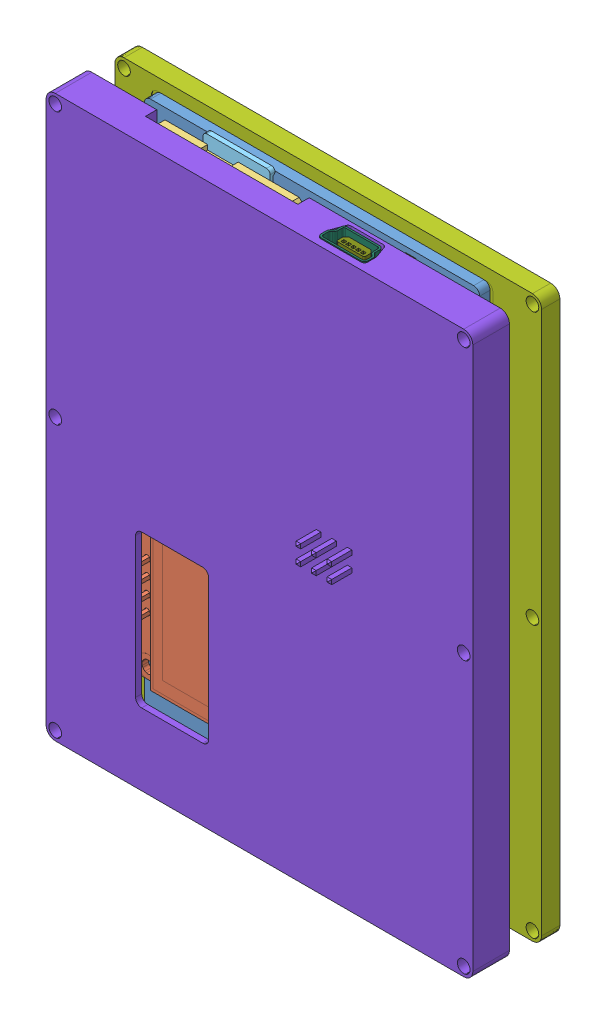
SolidWorks assembly Temperature & Humidity Meter, configuration Default. Lengths in mm.
Overall size (70.59 92.15 18.6).
51 component instances, 27 part files, 4 mates.
Components (placement in the parent):
- PCB.step-1: PCB.step [Default] at (27.42 35.7592 77.8723) size (55 92.15 18.6)
  - Board.step-1: Board.step [Default] at origin size (55 90 1.69)
    - Open CASCADE STEP translator 6.8 1.1.1.step-1: Open CASCADE STEP translator 6.8 1.1.1.step [Default] at (0 0 -1.6914) size (55 90 1.69)
  - O1.step-1: O1.step [Default] at origin size (27.98 26.7 10.85)
    - OLED_Display.step-1: OLED_Display.step [Default] at (-17.7739 15.5603 3.5437) x (0 1 0) z (0 0 1) size (26.7 27.98 10.85)
  - M1.step-1: M1.step [Default] at origin size (24 46.9 6.7)
    - MicroSD_Card.step-1: MicroSD_Card.step [Default] at (-7.7199 19.6 1.2127) x (0 -1 0) z (0 0 -1) size (46.9 24 6.7)
      - sdreader.step-1: sdreader.step [Default] at (-11.2744 2.632 -3.2) size (46.9 24 6.7)
        - Open CASCADE STEP translator 6.8 1.3.1.1.1.step-1: Open CASCADE STEP translator 6.8 1.3.1.1.1.step [Default] at origin size (46.9 24 6.7)
        - Open CASCADE STEP translator 6.8 1.3.1.1.2.step-1: Open CASCADE STEP translator 6.8 1.3.1.1.2.step [Default] at origin
      - AMS1117.step-1: AMS1117.step [Default] at (-0.4339 -2.128 -1.13) x (1 0 0) z (0 -1 0) size (6.51 1.86 7)
      - card_sd.step-1: card_sd.step [Default] at (-21.187 5.4466 -0.36) x (0 -1 0) z (0 0 1) size (11 15 0.82)
  - D1.step-1: D1.step [Default] at origin size (15.1 33.6 8.01)
    - DHT_22_RGB16777215.step-1: DHT_22_RGB16777215.step [Default] at (4.8899 -31.95 0.0126) x (1 0 0) z (0 0 1) size (15.1 33.6 8.01)
  - A1.step-1: A1.step [Default] at origin size (18 45.01 18.6)
    - Arduino_Nano.step-1: Arduino_Nano.step [Default] at (18.9901 8.2099 2.5126) x (0 1 0) z (1 0 0) size (45.01 18.6 18)
      - nano-board.step-1: nano-board.step [Default] at origin size (43.2 4.6 18)
      - 2pin_header__02.step-1: 2pin_header__02.step [Default] at (-1.143 1.6 -7.62) size (5 11.75 2.54)
      - 2pin_header__02.step-2: 2pin_header__02.step [Default] at (-1.143 1.6 -5.08) size (5 11.75 2.54)
      - 2pin_header__02.step-3: 2pin_header__02.step [Default] at (-1.143 1.6 -10.16) size (5 11.75 2.54)
      - 15pin_header__.step-1: 15pin_header__.step [Default] x (0 0 1) z (1 0 0) size (2.54 11.75 38.1)
      - 15pin_header__.step-2: 15pin_header__.step [Default] at (0 0 -15.24) x (0 0 1) z (1 0 0) size (2.54 11.75 38.1)
      - atmega328.step-1: atmega328.step [Default] at (23.85 1.75 -7.62) x (-0.707107 0 0.707107) z (-0.707107 0 -0.707107) size (10.01 1.11 10.01)
      - ftdi_FT232rl.step-1: ftdi_FT232rl.step [Default] at (29.05 0 -7.67) x (0 0 -1) z (-1 0 0) size (9.25 1.9 10.2)
      - smt_resistor222.step-1: smt_resistor222.step [Default] at (21.86 0 -5.8) x (0 0 -1) z (-1 0 0) size (1.7 0.6 3.8)
      - smt_resistor222.step-2: smt_resistor222.step [Default] at (21.86 0 -9) x (0 0 -1) z (-1 0 0) size (1.7 0.6 3.8)
      - smt_resistor222.step-3: smt_resistor222.step [Default] at (36.75 0 -7.6) x (0 0 -1) z (-1 0 0) size (1.7 0.6 3.8)
      - smt_resistor222.step-4: smt_resistor222.step [Default] at (36.75 0 -12) x (0 0 -1) z (-1 0 0) size (1.7 0.6 3.8)
      - smt_resistor222.step-5: smt_resistor222.step [Default] at (8.2 0 -2.6) x (0 0 -1) z (-1 0 0) size (1.7 0.6 3.8)
      - led.step-1: led.step [Default] at (10.4 1.6 -2.8) size (4.01 0.9 1.56)
      - led.step-2: led.step [Default] at (10.4 1.6 -5.55) size (4.01 0.9 1.56)
      - led.step-3: led.step [Default] at (10.4 1.6 -12.5) size (4.01 0.9 1.56)
      - led.step-4: led.step [Default] at (10.4 1.6 -9.05) size (4.01 0.9 1.56)
      - 16mhz_crystal_-_measured.step-1: 16mhz_crystal_-_measured.step [Default] at (18.5113 1.6 -3.5541) x (0.707107 0 0.707107) z (-0.707107 0 0.707107) size (3.4 0.8 2)
      - MINIUSBSHELL.step-1: MINIUSBSHELL.step [Default] at (38.98 1.65 -7.62) x (0 0 1) z (-1 0 0) size (10.9 3.77 9.41)
      - MINIUSBCORE.step-1: MINIUSBCORE.step [Default] at (32.28 1.65 -7.62) x (0 0 -1) z (1 0 0) size (7.7 4.5 8.2)
      - MINI_USB_CONTACT.step-1: MINI_USB_CONTACT.step [Default] at (33.28 1.65 -9.22) x (0 0 -1) z (1 0 0) size (0.5 2.55 9.42)
      - MINI_USB_CONTACT.step-2: MINI_USB_CONTACT.step [Default] at (33.28 1.65 -8.42) x (0 0 -1) z (1 0 0) size (0.5 2.55 9.42)
      - MINI_USB_CONTACT.step-3: MINI_USB_CONTACT.step [Default] at (33.28 1.65 -7.62) x (0 0 -1) z (1 0 0) size (0.5 2.55 9.42)
      - MINI_USB_CONTACT.step-4: MINI_USB_CONTACT.step [Default] at (33.28 1.65 -6.82) x (0 0 -1) z (1 0 0) size (0.5 2.55 9.42)
      - MINI_USB_CONTACT.step-5: MINI_USB_CONTACT.step [Default] at (33.28 1.65 -6.02) x (0 0 -1) z (1 0 0) size (0.5 2.55 9.42)
      - cap106C.step-1: cap106C.step [Default] at (37.2 0 -3.3) x (0 0 1) z (1 0 0) size (1.7 1.81 4)
      - cap106C.step-2: cap106C.step [Default] at (7.9 0 -5.6) x (0 0 -1) z (-1 0 0) size (1.7 1.81 4)
      - reset_core.step-1: reset_core.step [Default] at (15.25 1.6 -8.05) x (0 0 -1) z (1 0 0) size (5.21 2.15 2.8)
      - reset_shell.step-1: reset_shell.step [Default] at (15.25 3.25 -8.05) size (3 1.65 4)
      - nano_-_reg.step-1: nano_-_reg.step [Default] at (6.1 0 -10.16) x (0 0 -1) z (-1 0 0) size (6.5 1.69 8.3)
      - NANO_DIODE.step-1: NANO_DIODE.step [Default] at (11.43 0 -4.2) x (0 0 1) z (1 0 0) size (4.92 1.39 1.7)
      - 189_RESISTOR_PACK.step-1: 189_RESISTOR_PACK.step [Default] at (15.75 0 -10.85) x (0 0 1) z (1 0 0) size (3.2 0.51 3)
      - 102_RESISTOR_PACK.step-1: 102_RESISTOR_PACK.step [Default] at (15.75 0 -5.2) x (0 0 1) z (1 0 0) size (3.2 0.51 3)
- Enclosure Bottom-1: Enclosure Bottom [Default] at (27.1375 39.0102 76.1809) x (-1 0 0) z (0 0 -1) size (70 92 3)
- Enclosure top-2: Enclosure top [Default] at (26.5498 39.0102 86.8723) x (-1 0 0) z (0 0 -1) size (70 92 6)
Mates (geometry in assembly coordinates):
- Coincident16: coincident aligned: plane of PCB.step-1/Board.step-1/Open CASCADE STEP translator 6.8 1.1.1.step-1 through (52.683 -6.9898 76.1809) normal (0 -1 0); plane of Enclosure-1 through (60.6375 -6.9898 73.1809) normal (0 -1 0)
- Distance5: distance = 8 mm anti-aligned: plane of PCB.step-1/Board.step-1/Open CASCADE STEP translator 6.8 1.1.1.step-1 through (-1.317 -5.9898 77.8723) normal (0 0 1); plane of Enclosure top-2 through (-6.9502 83.5102 85.8723) normal (0 0 -1)
- Coincident19: coincident aligned: plane of Enclosure-1 through (60.6375 -6.9898 73.1809) normal (0 -1 0); plane of Enclosure top-2 through (60.0498 -6.9898 85.8723) normal (0 -1 0)
- Coincident22: coincident anti-aligned: plane of PCB.step-1/Board.step-1/Open CASCADE STEP translator 6.8 1.1.1.step-1 through (-1.317 -5.9898 76.1809) normal (0 0 -1); plane of Enclosure-1 through (-6.3625 83.5102 76.1809) normal (0 0 1)
